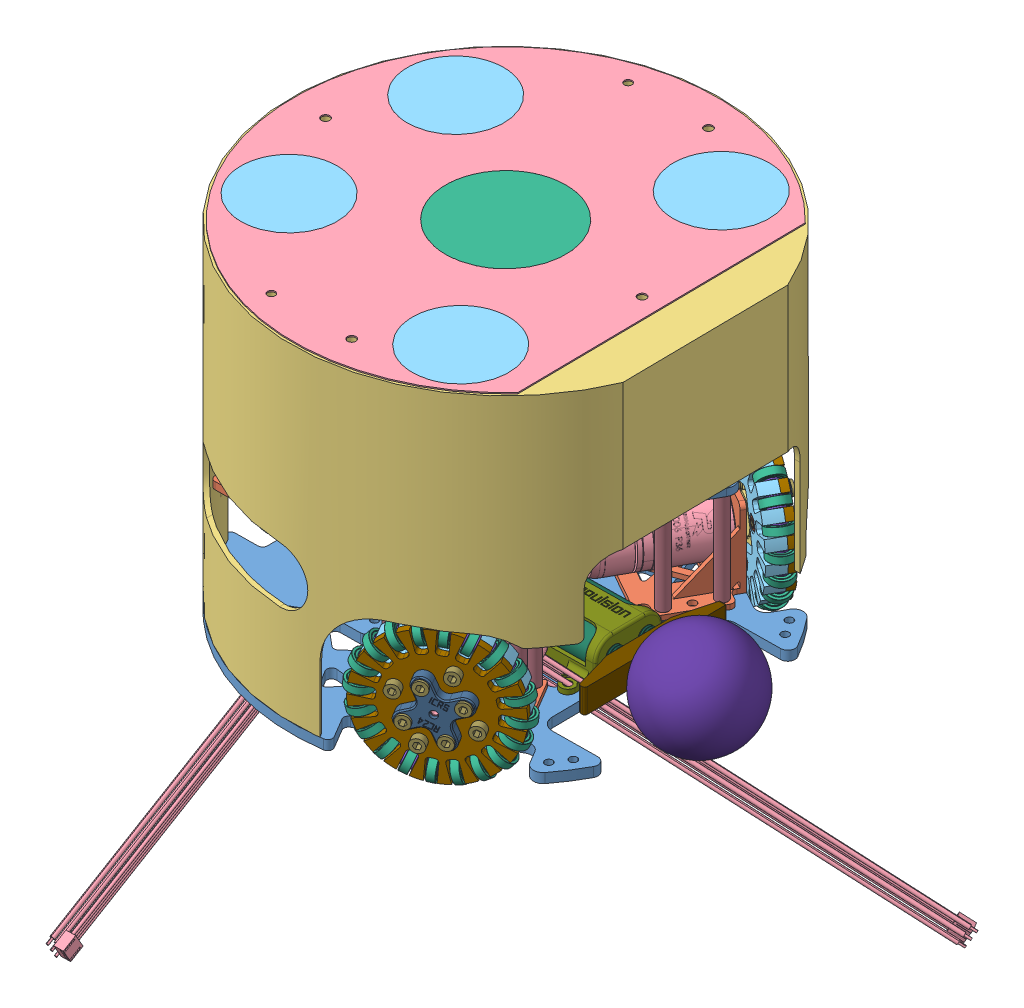
SolidWorks assembly ASM_ICRS_RCssl_2024_drive_base_Tri_wheel-intermediate, configuration Default. Lengths in mm.
Overall size (302.45 245.12 306.72).
392 component instances, 24 part files, 44 mates.
Components (placement in the parent):
- CF4mm_RCssl_drive_base_ground_Tri_wheel-1: CF4mm_RCssl_drive_base_ground_Tri_wheel [Default] at (-0.754 -4 -10.7249) x (-0.011698 0 -0.999932) z (0 1 0) size (182.55 180 57.77)
- RCSSL_gen2_OW_drive_unit-1: RCSSL_gen2_OW_drive_unit [Default] at (35.2509 -22.9667 -96.722) x (0.871815 0 0.489835) z (-0.489835 0 0.871815) size (193.31 168.77 67.31)
  - 1.5mm_aluminium_metal_plating_2006 motor mount-1: 1.5mm_aluminium_metal_plating_2006 motor mount [Default] at (10.7348 39.9667 23.6101) size (46 32 35)
  - 3dp_AL_Gen2_Customised_AL_shaft_flange_connector_2006-1: 3dp_AL_Gen2_Customised_AL_shaft_flange_connector_2006 [Default] at (10.7348 39.9667 8.6101) x (0.866025 0.5 0) z (0 0 1) size (34 34 12.5)
  - RoboMaster M2006 P36 motor 1-1: RoboMaster M2006 P36 motor 1 [默认] at (29.0021 49.1921 55.5053) x (0.258819 0.965926 0) z (0 0 1) size (137.53 138.78 64.81)
  - ASM_RCssl_OW_Ver2-1: ASM_RCssl_OW_Ver2 [Default] at (25.0097 83.9716 -12.1645) x (-0.924615 -0.380903 0) z (0 0 1) size (59.33 59.33 15) (flexible)
    - 3dp_PETG_RCssl_OW_ver2_base-1: 3dp_PETG_RCssl_OW_ver2_base [Default] at (29.9603 35.2502 26.2746) size (54.84 54.84 7)
    - RCssl_OW_Ver2_roller_bearing_ASM-1: RCssl_OW_Ver2_roller_bearing_ASM [Default] at (24.4121 54.6156 21.3003) x (0 1 0) z (1 0 0) size (10 10 6)
      - BK_PU_68_3_10_3_bearing+roller-1: BK_PU_68_3_10_3_bearing+roller [Default] at (5.2981 6.4743 4.0482) size (10 10 3)
      - D3_H6_mid_axis-1: D3_H6_mid_axis [Default] at (5.2981 6.4743 2.5482) size (2.96 2.96 6)
      - m3_D6_H0.5_washer-1: m3_D6_H0.5_washer [Default] at (5.2981 6.4743 3.5482) x (0.872248 -0.489064 0) z (0 0 1) size (6 6 0.5)
      - m3_D6_H0.5_washer-2: m3_D6_H0.5_washer [Default] at (5.2981 6.4743 7.0482) size (6 6 0.5)
    - RCssl_OW_Ver2_roller_bearing_ASM-2: RCssl_OW_Ver2_roller_bearing_ASM [Default] at (30.6679 55.3823 21.3003) x (0.309017 0.951057 0) z (0.951057 -0.309017 0) size (10 10 6)
      - BK_PU_68_3_10_3_bearing+roller-1: BK_PU_68_3_10_3_bearing+roller [Default] at (5.2981 6.4743 4.0482) size (10 10 3)
      - D3_H6_mid_axis-1: D3_H6_mid_axis [Default] at (5.2981 6.4743 2.5482) size (2.96 2.96 6)
      - m3_D6_H0.5_washer-1: m3_D6_H0.5_washer [Default] at (5.2981 6.4743 3.5482) x (0.872248 -0.489064 0) z (0 0 1) size (6 6 0.5)
      - m3_D6_H0.5_washer-2: m3_D6_H0.5_washer [Default] at (5.2981 6.4743 7.0482) size (6 6 0.5)
    - RCssl_OW_Ver2_roller_bearing_ASM-3: RCssl_OW_Ver2_roller_bearing_ASM [Default] at (36.8544 54.1783 21.3003) x (0.587785 0.809017 0) z (0.809017 -0.587785 0) size (10 10 6)
      - BK_PU_68_3_10_3_bearing+roller-1: BK_PU_68_3_10_3_bearing+roller [Default] at (5.2981 6.4743 4.0482) size (10 10 3)
      - D3_H6_mid_axis-1: D3_H6_mid_axis [Default] at (5.2981 6.4743 2.5482) size (2.96 2.96 6)
      - m3_D6_H0.5_washer-1: m3_D6_H0.5_washer [Default] at (5.2981 6.4743 3.5482) x (0.872248 -0.489064 0) z (0 0 1) size (6 6 0.5)
      - m3_D6_H0.5_washer-2: m3_D6_H0.5_washer [Default] at (5.2981 6.4743 7.0482) size (6 6 0.5)
    - RCssl_OW_Ver2_roller_bearing_ASM-4: RCssl_OW_Ver2_roller_bearing_ASM [Default] at (42.3661 51.1215 21.3003) x (0.809017 0.587785 0) z (0.587785 -0.809017 0) size (10 10 6)
      - BK_PU_68_3_10_3_bearing+roller-1: BK_PU_68_3_10_3_bearing+roller [Default] at (5.2981 6.4743 4.0482) size (10 10 3)
      - D3_H6_mid_axis-1: D3_H6_mid_axis [Default] at (5.2981 6.4743 2.5482) size (2.96 2.96 6)
      - m3_D6_H0.5_washer-1: m3_D6_H0.5_washer [Default] at (5.2981 6.4743 3.5482) x (0.872248 -0.489064 0) z (0 0 1) size (6 6 0.5)
      - m3_D6_H0.5_washer-2: m3_D6_H0.5_washer [Default] at (5.2981 6.4743 7.0482) size (6 6 0.5)
    - RCssl_OW_Ver2_roller_bearing_ASM-5: RCssl_OW_Ver2_roller_bearing_ASM [Default] at (46.6634 46.5111 21.3003) x (0.951057 0.309017 0) z (0.309017 -0.951057 0) size (10 10 6)
      - BK_PU_68_3_10_3_bearing+roller-1: BK_PU_68_3_10_3_bearing+roller [Default] at (5.2981 6.4743 4.0482) size (10 10 3)
      - D3_H6_mid_axis-1: D3_H6_mid_axis [Default] at (5.2981 6.4743 2.5482) size (2.96 2.96 6)
      - m3_D6_H0.5_washer-1: m3_D6_H0.5_washer [Default] at (5.2981 6.4743 3.5482) x (0.872248 -0.489064 0) z (0 0 1) size (6 6 0.5)
      - m3_D6_H0.5_washer-2: m3_D6_H0.5_washer [Default] at (5.2981 6.4743 7.0482) size (6 6 0.5)
    - RCssl_OW_Ver2_roller_bearing_ASM-6: RCssl_OW_Ver2_roller_bearing_ASM [Default] at (49.3257 40.7985 21.3003) x (1 0 0) z (0 -1 0) size (10 10 6)
      - BK_PU_68_3_10_3_bearing+roller-1: BK_PU_68_3_10_3_bearing+roller [Default] at (5.2981 6.4743 4.0482) size (10 10 3)
      - D3_H6_mid_axis-1: D3_H6_mid_axis [Default] at (5.2981 6.4743 2.5482) size (2.96 2.96 6)
      - m3_D6_H0.5_washer-1: m3_D6_H0.5_washer [Default] at (5.2981 6.4743 3.5482) x (0.872248 -0.489064 0) z (0 0 1) size (6 6 0.5)
      - m3_D6_H0.5_washer-2: m3_D6_H0.5_washer [Default] at (5.2981 6.4743 7.0482) size (6 6 0.5)
    - RCssl_OW_Ver2_roller_bearing_ASM-7: RCssl_OW_Ver2_roller_bearing_ASM [Default] at (50.0924 34.5427 21.3003) x (0.951057 -0.309017 0) z (-0.309017 -0.951057 0) size (10 10 6)
      - BK_PU_68_3_10_3_bearing+roller-1: BK_PU_68_3_10_3_bearing+roller [Default] at (5.2981 6.4743 4.0482) size (10 10 3)
      - D3_H6_mid_axis-1: D3_H6_mid_axis [Default] at (5.2981 6.4743 2.5482) size (2.96 2.96 6)
      - m3_D6_H0.5_washer-1: m3_D6_H0.5_washer [Default] at (5.2981 6.4743 3.5482) x (0.872248 -0.489064 0) z (0 0 1) size (6 6 0.5)
      - m3_D6_H0.5_washer-2: m3_D6_H0.5_washer [Default] at (5.2981 6.4743 7.0482) size (6 6 0.5)
    - RCssl_OW_Ver2_roller_bearing_ASM-8: RCssl_OW_Ver2_roller_bearing_ASM [Default] at (48.8884 28.3562 21.3003) x (0.809017 -0.587785 0) z (-0.587785 -0.809017 0) size (10 10 6)
      - BK_PU_68_3_10_3_bearing+roller-1: BK_PU_68_3_10_3_bearing+roller [Default] at (5.2981 6.4743 4.0482) size (10 10 3)
      - D3_H6_mid_axis-1: D3_H6_mid_axis [Default] at (5.2981 6.4743 2.5482) size (2.96 2.96 6)
      - m3_D6_H0.5_washer-1: m3_D6_H0.5_washer [Default] at (5.2981 6.4743 3.5482) x (0.872248 -0.489064 0) z (0 0 1) size (6 6 0.5)
      - m3_D6_H0.5_washer-2: m3_D6_H0.5_washer [Default] at (5.2981 6.4743 7.0482) size (6 6 0.5)
    - RCssl_OW_Ver2_roller_bearing_ASM-9: RCssl_OW_Ver2_roller_bearing_ASM [Default] at (45.8316 22.8445 21.3003) x (0.587785 -0.809017 0) z (-0.809017 -0.587785 0) size (10 10 6)
      - BK_PU_68_3_10_3_bearing+roller-1: BK_PU_68_3_10_3_bearing+roller [Default] at (5.2981 6.4743 4.0482) size (10 10 3)
      - D3_H6_mid_axis-1: D3_H6_mid_axis [Default] at (5.2981 6.4743 2.5482) size (2.96 2.96 6)
      - m3_D6_H0.5_washer-1: m3_D6_H0.5_washer [Default] at (5.2981 6.4743 3.5482) x (0.872248 -0.489064 0) z (0 0 1) size (6 6 0.5)
      - m3_D6_H0.5_washer-2: m3_D6_H0.5_washer [Default] at (5.2981 6.4743 7.0482) size (6 6 0.5)
    - RCssl_OW_Ver2_roller_bearing_ASM-10: RCssl_OW_Ver2_roller_bearing_ASM [Default] at (41.2212 18.5472 21.3003) x (0.309017 -0.951057 0) z (-0.951057 -0.309017 0) size (10 10 6)
      - BK_PU_68_3_10_3_bearing+roller-1: BK_PU_68_3_10_3_bearing+roller [Default] at (5.2981 6.4743 4.0482) size (10 10 3)
      - D3_H6_mid_axis-1: D3_H6_mid_axis [Default] at (5.2981 6.4743 2.5482) size (2.96 2.96 6)
      - m3_D6_H0.5_washer-1: m3_D6_H0.5_washer [Default] at (5.2981 6.4743 3.5482) x (0.872248 -0.489064 0) z (0 0 1) size (6 6 0.5)
      - m3_D6_H0.5_washer-2: m3_D6_H0.5_washer [Default] at (5.2981 6.4743 7.0482) size (6 6 0.5)
    - RCssl_OW_Ver2_roller_bearing_ASM-11: RCssl_OW_Ver2_roller_bearing_ASM [Default] at (35.5086 15.8849 21.3003) x (0 -1 0) z (-1 0 0) size (10 10 6)
      - BK_PU_68_3_10_3_bearing+roller-1: BK_PU_68_3_10_3_bearing+roller [Default] at (5.2981 6.4743 4.0482) size (10 10 3)
      - D3_H6_mid_axis-1: D3_H6_mid_axis [Default] at (5.2981 6.4743 2.5482) size (2.96 2.96 6)
      - m3_D6_H0.5_washer-1: m3_D6_H0.5_washer [Default] at (5.2981 6.4743 3.5482) x (0.872248 -0.489064 0) z (0 0 1) size (6 6 0.5)
      - m3_D6_H0.5_washer-2: m3_D6_H0.5_washer [Default] at (5.2981 6.4743 7.0482) size (6 6 0.5)
    - RCssl_OW_Ver2_roller_bearing_ASM-12: RCssl_OW_Ver2_roller_bearing_ASM [Default] at (29.2528 15.1182 21.3003) x (-0.309017 -0.951057 0) z (-0.951057 0.309017 0) size (10 10 6)
      - BK_PU_68_3_10_3_bearing+roller-1: BK_PU_68_3_10_3_bearing+roller [Default] at (5.2981 6.4743 4.0482) size (10 10 3)
      - D3_H6_mid_axis-1: D3_H6_mid_axis [Default] at (5.2981 6.4743 2.5482) size (2.96 2.96 6)
      - m3_D6_H0.5_washer-1: m3_D6_H0.5_washer [Default] at (5.2981 6.4743 3.5482) x (0.872248 -0.489064 0) z (0 0 1) size (6 6 0.5)
      - m3_D6_H0.5_washer-2: m3_D6_H0.5_washer [Default] at (5.2981 6.4743 7.0482) size (6 6 0.5)
    - RCssl_OW_Ver2_roller_bearing_ASM-13: RCssl_OW_Ver2_roller_bearing_ASM [Default] at (23.0663 16.3222 21.3003) x (-0.587785 -0.809017 0) z (-0.809017 0.587785 0) size (10 10 6)
      - BK_PU_68_3_10_3_bearing+roller-1: BK_PU_68_3_10_3_bearing+roller [Default] at (5.2981 6.4743 4.0482) size (10 10 3)
      - D3_H6_mid_axis-1: D3_H6_mid_axis [Default] at (5.2981 6.4743 2.5482) size (2.96 2.96 6)
      - m3_D6_H0.5_washer-1: m3_D6_H0.5_washer [Default] at (5.2981 6.4743 3.5482) x (0.872248 -0.489064 0) z (0 0 1) size (6 6 0.5)
      - m3_D6_H0.5_washer-2: m3_D6_H0.5_washer [Default] at (5.2981 6.4743 7.0482) size (6 6 0.5)
    - RCssl_OW_Ver2_roller_bearing_ASM-14: RCssl_OW_Ver2_roller_bearing_ASM [Default] at (17.5546 19.379 21.3003) x (-0.809017 -0.587785 0) z (-0.587785 0.809017 0) size (10 10 6)
      - BK_PU_68_3_10_3_bearing+roller-1: BK_PU_68_3_10_3_bearing+roller [Default] at (5.2981 6.4743 4.0482) size (10 10 3)
      - D3_H6_mid_axis-1: D3_H6_mid_axis [Default] at (5.2981 6.4743 2.5482) size (2.96 2.96 6)
      - m3_D6_H0.5_washer-1: m3_D6_H0.5_washer [Default] at (5.2981 6.4743 3.5482) x (0.872248 -0.489064 0) z (0 0 1) size (6 6 0.5)
      - m3_D6_H0.5_washer-2: m3_D6_H0.5_washer [Default] at (5.2981 6.4743 7.0482) size (6 6 0.5)
    - RCssl_OW_Ver2_roller_bearing_ASM-15: RCssl_OW_Ver2_roller_bearing_ASM [Default] at (13.2573 23.9893 21.3003) x (-0.951057 -0.309017 0) z (-0.309017 0.951057 0) size (10 10 6)
      - BK_PU_68_3_10_3_bearing+roller-1: BK_PU_68_3_10_3_bearing+roller [Default] at (5.2981 6.4743 4.0482) size (10 10 3)
      - D3_H6_mid_axis-1: D3_H6_mid_axis [Default] at (5.2981 6.4743 2.5482) size (2.96 2.96 6)
      - m3_D6_H0.5_washer-1: m3_D6_H0.5_washer [Default] at (5.2981 6.4743 3.5482) x (0.872248 -0.489064 0) z (0 0 1) size (6 6 0.5)
      - m3_D6_H0.5_washer-2: m3_D6_H0.5_washer [Default] at (5.2981 6.4743 7.0482) size (6 6 0.5)
    - RCssl_OW_Ver2_roller_bearing_ASM-16: RCssl_OW_Ver2_roller_bearing_ASM [Default] at (10.595 29.702 21.3003) x (-1 0 0) z (0 1 0) size (10 10 6)
      - BK_PU_68_3_10_3_bearing+roller-1: BK_PU_68_3_10_3_bearing+roller [Default] at (5.2981 6.4743 4.0482) size (10 10 3)
      - D3_H6_mid_axis-1: D3_H6_mid_axis [Default] at (5.2981 6.4743 2.5482) size (2.96 2.96 6)
      - m3_D6_H0.5_washer-1: m3_D6_H0.5_washer [Default] at (5.2981 6.4743 3.5482) x (0.872248 -0.489064 0) z (0 0 1) size (6 6 0.5)
      - m3_D6_H0.5_washer-2: m3_D6_H0.5_washer [Default] at (5.2981 6.4743 7.0482) size (6 6 0.5)
    - RCssl_OW_Ver2_roller_bearing_ASM-17: RCssl_OW_Ver2_roller_bearing_ASM [Default] at (9.8283 35.9578 21.3003) x (-0.951057 0.309017 0) z (0.309017 0.951057 0) size (10 10 6)
      - BK_PU_68_3_10_3_bearing+roller-1: BK_PU_68_3_10_3_bearing+roller [Default] at (5.2981 6.4743 4.0482) size (10 10 3)
      - D3_H6_mid_axis-1: D3_H6_mid_axis [Default] at (5.2981 6.4743 2.5482) size (2.96 2.96 6)
      - m3_D6_H0.5_washer-1: m3_D6_H0.5_washer [Default] at (5.2981 6.4743 3.5482) x (0.872248 -0.489064 0) z (0 0 1) size (6 6 0.5)
      - m3_D6_H0.5_washer-2: m3_D6_H0.5_washer [Default] at (5.2981 6.4743 7.0482) size (6 6 0.5)
    - RCssl_OW_Ver2_roller_bearing_ASM-18: RCssl_OW_Ver2_roller_bearing_ASM [Default] at (11.0323 42.1443 21.3003) x (-0.809017 0.587785 0) z (0.587785 0.809017 0) size (10 10 6)
      - BK_PU_68_3_10_3_bearing+roller-1: BK_PU_68_3_10_3_bearing+roller [Default] at (5.2981 6.4743 4.0482) size (10 10 3)
      - D3_H6_mid_axis-1: D3_H6_mid_axis [Default] at (5.2981 6.4743 2.5482) size (2.96 2.96 6)
      - m3_D6_H0.5_washer-1: m3_D6_H0.5_washer [Default] at (5.2981 6.4743 3.5482) x (0.872248 -0.489064 0) z (0 0 1) size (6 6 0.5)
      - m3_D6_H0.5_washer-2: m3_D6_H0.5_washer [Default] at (5.2981 6.4743 7.0482) size (6 6 0.5)
    - RCssl_OW_Ver2_roller_bearing_ASM-19: RCssl_OW_Ver2_roller_bearing_ASM [Default] at (14.0891 47.656 21.3003) x (-0.587785 0.809017 0) z (0.809017 0.587785 0) size (10 10 6) (flexible)
      - BK_PU_68_3_10_3_bearing+roller-1: BK_PU_68_3_10_3_bearing+roller [Default] at (5.2981 6.4743 4.0482) size (10 10 3)
      - D3_H6_mid_axis-1: D3_H6_mid_axis [Default] at (5.2981 6.4743 2.5482) size (2.96 2.96 6)
      - m3_D6_H0.5_washer-1: m3_D6_H0.5_washer [Default] at (5.2981 6.4743 3.5482) x (0.872248 -0.489064 0) z (0 0 1) size (6 6 0.5)
      - m3_D6_H0.5_washer-2: m3_D6_H0.5_washer [Default] at (5.2981 6.4743 7.0482) size (6 6 0.5)
    - RCssl_OW_Ver2_roller_bearing_ASM-20: RCssl_OW_Ver2_roller_bearing_ASM [Default] at (18.6994 51.9533 21.3003) x (-0.309017 0.951057 0) z (0.951057 0.309017 0) size (10 10 6)
      - BK_PU_68_3_10_3_bearing+roller-1: BK_PU_68_3_10_3_bearing+roller [Default] at (5.2981 6.4743 4.0482) size (10 10 3)
      - D3_H6_mid_axis-1: D3_H6_mid_axis [Default] at (5.2981 6.4743 2.5482) size (2.96 2.96 6)
      - m3_D6_H0.5_washer-1: m3_D6_H0.5_washer [Default] at (5.2981 6.4743 3.5482) x (0.872248 -0.489064 0) z (0 0 1) size (6 6 0.5)
      - m3_D6_H0.5_washer-2: m3_D6_H0.5_washer [Default] at (5.2981 6.4743 7.0482) size (6 6 0.5)
    - CF3mm_OW_gen2_output_plane-1: CF3mm_OW_gen2_output_plane [Default] at (29.9603 35.2502 44.7746) size (54.84 54.84 3)
    - 3dp_PETG_RCssl_OW_front_lock-1: 3dp_PETG_RCssl_OW_front_lock [Default] at (29.9603 35.2502 21.2746) x (1 0 0) z (0 0 -1) size (21.15 21.15 4.13)
    - nut_din_985-m3x0_5-8-1: nut_din_985-m3x0_5-8 [Default] at (29.9603 21.2502 29.2746) x (-1 0 0) z (0 0 -1) size (6.2 5.5 4)
    - nut_din_985-m3x0_5-8-2: nut_din_985-m3x0_5-8 [Default] at (15.9603 35.2502 29.2746) x (0 1 0) z (0 0 -1) size (6.2 5.5 4)
    - nut_din_985-m3x0_5-8-3: nut_din_985-m3x0_5-8 [Default] at (29.9603 49.2502 29.2746) x (1 0 0) z (0 0 -1) size (6.2 5.5 4)
    - nut_din_985-m3x0_5-8-4: nut_din_985-m3x0_5-8 [Default] at (43.9603 35.2502 29.2746) x (0 -1 0) z (0 0 -1) size (6.2 5.5 4)
    - M3_304__full_teeth__screw_10mm-1: M3_304__full_teeth__screw_10mm [Default] at (29.992 49.2503 23.2746) x (-0.002323 0.999997 0) z (0 0 -1) size (5.3 5.3 13)
    - M3_304__full_teeth__screw_10mm-2: M3_304__full_teeth__screw_10mm [Default] at (43.9604 35.2186 23.2746) x (0.999997 0.002323 0) z (0 0 -1) size (5.3 5.3 13)
    - M3_304__full_teeth__screw_10mm-3: M3_304__full_teeth__screw_10mm [Default] at (29.9287 21.2502 23.2746) x (0.002323 -0.999997 0) z (0 0 -1) size (5.3 5.3 13)
    - M3_304__full_teeth__screw_10mm-4: M3_304__full_teeth__screw_10mm [Default] at (15.9603 35.2819 23.2746) x (-0.999997 -0.002323 0) z (0 0 -1) size (5.3 5.3 13)
    - M3_304__full_teeth__screw_10mm-5: M3_304__full_teeth__screw_10mm [Default] at (37.0442 42.2923 21.2746) x (0.914728 0.40407 0) z (0 0 -1) size (5.3 5.3 13)
    - M3_304__full_teeth__screw_10mm-6: M3_304__full_teeth__screw_10mm [Default] at (37.0024 28.1664 21.2746) x (0.40407 -0.914728 0) z (0 0 -1) size (5.3 5.3 13)
    - M3_304__full_teeth__screw_10mm-7: M3_304__full_teeth__screw_10mm [Default] at (22.8765 28.2081 21.2746) x (-0.914728 -0.40407 0) z (0 0 -1) size (5.3 5.3 13)
    - M3_304__full_teeth__screw_10mm-8: M3_304__full_teeth__screw_10mm [Default] at (22.9182 42.3341 21.2746) x (-0.40407 0.914728 0) z (0 0 -1) size (5.3 5.3 13)
  - AL_pillar_M3_D6_H40_Threaded-2: AL_pillar_M3_D6_H40_Threaded [H30] at (-8.7652 24.9667 50.1101) size (5 40 5)
  - AL_pillar_M3_D6_H40_Threaded-3: AL_pillar_M3_D6_H40_Threaded [H30] at (30.2348 24.9667 50.1101) size (5 40 5)
  - AL_pillar_M3_D6_H40_Threaded-4: AL_pillar_M3_D6_H40_Threaded [Default] at (30.2348 24.9667 32.1101) x (0.546545 0 0.83743) z (-0.83743 0 0.546545) size (5 40 5)
  - AL_pillar_M3_D6_H40_Threaded-5: AL_pillar_M3_D6_H40_Threaded [Default] at (-8.7652 24.9667 32.1101) x (0.546545 0 0.83743) z (-0.83743 0 0.546545) size (5 40 5)
- RCSSL_gen2_OW_drive_unit-2: RCSSL_gen2_OW_drive_unit [Default] at (55.7193 -22.9667 63.4549) x (-0.860117 0 0.510097) z (-0.510097 0 -0.860117) size (193.31 168.77 67.31)
  - 1.5mm_aluminium_metal_plating_2006 motor mount-1: 1.5mm_aluminium_metal_plating_2006 motor mount [Default] at (10.7348 39.9667 23.6101) size (46 32 35)
  - 3dp_AL_Gen2_Customised_AL_shaft_flange_connector_2006-1: 3dp_AL_Gen2_Customised_AL_shaft_flange_connector_2006 [Default] at (10.7348 39.9667 8.6101) x (0.866025 0.5 0) z (0 0 1) size (34 34 12.5)
  - RoboMaster M2006 P36 motor 1-1: RoboMaster M2006 P36 motor 1 [默认] at (29.0021 49.1921 55.5053) x (0.258819 0.965926 0) z (0 0 1) size (137.53 138.78 64.81)
  - ASM_RCssl_OW_Ver2-1: ASM_RCssl_OW_Ver2 [Default] at (25.0097 83.9716 -12.1645) x (-0.924615 -0.380903 0) z (0 0 1) size (59.33 59.33 15) (flexible)
    - 3dp_PETG_RCssl_OW_ver2_base-1: 3dp_PETG_RCssl_OW_ver2_base [Default] at (29.9603 35.2502 26.2746) size (54.84 54.84 7)
    - RCssl_OW_Ver2_roller_bearing_ASM-1: RCssl_OW_Ver2_roller_bearing_ASM [Default] at (24.4121 54.6156 21.3003) x (0 1 0) z (1 0 0) size (10 10 6)
      - BK_PU_68_3_10_3_bearing+roller-1: BK_PU_68_3_10_3_bearing+roller [Default] at (5.2981 6.4743 4.0482) size (10 10 3)
      - D3_H6_mid_axis-1: D3_H6_mid_axis [Default] at (5.2981 6.4743 2.5482) size (2.96 2.96 6)
      - m3_D6_H0.5_washer-1: m3_D6_H0.5_washer [Default] at (5.2981 6.4743 3.5482) x (0.872248 -0.489064 0) z (0 0 1) size (6 6 0.5)
      - m3_D6_H0.5_washer-2: m3_D6_H0.5_washer [Default] at (5.2981 6.4743 7.0482) size (6 6 0.5)
    - RCssl_OW_Ver2_roller_bearing_ASM-2: RCssl_OW_Ver2_roller_bearing_ASM [Default] at (30.6679 55.3823 21.3003) x (0.309017 0.951057 0) z (0.951057 -0.309017 0) size (10 10 6)
      - BK_PU_68_3_10_3_bearing+roller-1: BK_PU_68_3_10_3_bearing+roller [Default] at (5.2981 6.4743 4.0482) size (10 10 3)
      - D3_H6_mid_axis-1: D3_H6_mid_axis [Default] at (5.2981 6.4743 2.5482) size (2.96 2.96 6)
      - m3_D6_H0.5_washer-1: m3_D6_H0.5_washer [Default] at (5.2981 6.4743 3.5482) x (0.872248 -0.489064 0) z (0 0 1) size (6 6 0.5)
      - m3_D6_H0.5_washer-2: m3_D6_H0.5_washer [Default] at (5.2981 6.4743 7.0482) size (6 6 0.5)
    - RCssl_OW_Ver2_roller_bearing_ASM-3: RCssl_OW_Ver2_roller_bearing_ASM [Default] at (36.8544 54.1783 21.3003) x (0.587785 0.809017 0) z (0.809017 -0.587785 0) size (10 10 6)
      - BK_PU_68_3_10_3_bearing+roller-1: BK_PU_68_3_10_3_bearing+roller [Default] at (5.2981 6.4743 4.0482) size (10 10 3)
      - D3_H6_mid_axis-1: D3_H6_mid_axis [Default] at (5.2981 6.4743 2.5482) size (2.96 2.96 6)
      - m3_D6_H0.5_washer-1: m3_D6_H0.5_washer [Default] at (5.2981 6.4743 3.5482) x (0.872248 -0.489064 0) z (0 0 1) size (6 6 0.5)
      - m3_D6_H0.5_washer-2: m3_D6_H0.5_washer [Default] at (5.2981 6.4743 7.0482) size (6 6 0.5)
    - RCssl_OW_Ver2_roller_bearing_ASM-4: RCssl_OW_Ver2_roller_bearing_ASM [Default] at (42.3661 51.1215 21.3003) x (0.809017 0.587785 0) z (0.587785 -0.809017 0) size (10 10 6)
      - BK_PU_68_3_10_3_bearing+roller-1: BK_PU_68_3_10_3_bearing+roller [Default] at (5.2981 6.4743 4.0482) size (10 10 3)
      - D3_H6_mid_axis-1: D3_H6_mid_axis [Default] at (5.2981 6.4743 2.5482) size (2.96 2.96 6)
      - m3_D6_H0.5_washer-1: m3_D6_H0.5_washer [Default] at (5.2981 6.4743 3.5482) x (0.872248 -0.489064 0) z (0 0 1) size (6 6 0.5)
      - m3_D6_H0.5_washer-2: m3_D6_H0.5_washer [Default] at (5.2981 6.4743 7.0482) size (6 6 0.5)
    - RCssl_OW_Ver2_roller_bearing_ASM-5: RCssl_OW_Ver2_roller_bearing_ASM [Default] at (46.6634 46.5111 21.3003) x (0.951057 0.309017 0) z (0.309017 -0.951057 0) size (10 10 6)
      - BK_PU_68_3_10_3_bearing+roller-1: BK_PU_68_3_10_3_bearing+roller [Default] at (5.2981 6.4743 4.0482) size (10 10 3)
      - D3_H6_mid_axis-1: D3_H6_mid_axis [Default] at (5.2981 6.4743 2.5482) size (2.96 2.96 6)
      - m3_D6_H0.5_washer-1: m3_D6_H0.5_washer [Default] at (5.2981 6.4743 3.5482) x (0.872248 -0.489064 0) z (0 0 1) size (6 6 0.5)
      - m3_D6_H0.5_washer-2: m3_D6_H0.5_washer [Default] at (5.2981 6.4743 7.0482) size (6 6 0.5)
    - RCssl_OW_Ver2_roller_bearing_ASM-6: RCssl_OW_Ver2_roller_bearing_ASM [Default] at (49.3257 40.7985 21.3003) x (1 0 0) z (0 -1 0) size (10 10 6)
      - BK_PU_68_3_10_3_bearing+roller-1: BK_PU_68_3_10_3_bearing+roller [Default] at (5.2981 6.4743 4.0482) size (10 10 3)
      - D3_H6_mid_axis-1: D3_H6_mid_axis [Default] at (5.2981 6.4743 2.5482) size (2.96 2.96 6)
      - m3_D6_H0.5_washer-1: m3_D6_H0.5_washer [Default] at (5.2981 6.4743 3.5482) x (0.872248 -0.489064 0) z (0 0 1) size (6 6 0.5)
      - m3_D6_H0.5_washer-2: m3_D6_H0.5_washer [Default] at (5.2981 6.4743 7.0482) size (6 6 0.5)
    - RCssl_OW_Ver2_roller_bearing_ASM-7: RCssl_OW_Ver2_roller_bearing_ASM [Default] at (50.0924 34.5427 21.3003) x (0.951057 -0.309017 0) z (-0.309017 -0.951057 0) size (10 10 6)
      - BK_PU_68_3_10_3_bearing+roller-1: BK_PU_68_3_10_3_bearing+roller [Default] at (5.2981 6.4743 4.0482) size (10 10 3)
      - D3_H6_mid_axis-1: D3_H6_mid_axis [Default] at (5.2981 6.4743 2.5482) size (2.96 2.96 6)
      - m3_D6_H0.5_washer-1: m3_D6_H0.5_washer [Default] at (5.2981 6.4743 3.5482) x (0.872248 -0.489064 0) z (0 0 1) size (6 6 0.5)
      - m3_D6_H0.5_washer-2: m3_D6_H0.5_washer [Default] at (5.2981 6.4743 7.0482) size (6 6 0.5)
    - RCssl_OW_Ver2_roller_bearing_ASM-8: RCssl_OW_Ver2_roller_bearing_ASM [Default] at (48.8884 28.3562 21.3003) x (0.809017 -0.587785 0) z (-0.587785 -0.809017 0) size (10 10 6)
      - BK_PU_68_3_10_3_bearing+roller-1: BK_PU_68_3_10_3_bearing+roller [Default] at (5.2981 6.4743 4.0482) size (10 10 3)
      - D3_H6_mid_axis-1: D3_H6_mid_axis [Default] at (5.2981 6.4743 2.5482) size (2.96 2.96 6)
      - m3_D6_H0.5_washer-1: m3_D6_H0.5_washer [Default] at (5.2981 6.4743 3.5482) x (0.872248 -0.489064 0) z (0 0 1) size (6 6 0.5)
      - m3_D6_H0.5_washer-2: m3_D6_H0.5_washer [Default] at (5.2981 6.4743 7.0482) size (6 6 0.5)
    - RCssl_OW_Ver2_roller_bearing_ASM-9: RCssl_OW_Ver2_roller_bearing_ASM [Default] at (45.8316 22.8445 21.3003) x (0.587785 -0.809017 0) z (-0.809017 -0.587785 0) size (10 10 6)
      - BK_PU_68_3_10_3_bearing+roller-1: BK_PU_68_3_10_3_bearing+roller [Default] at (5.2981 6.4743 4.0482) size (10 10 3)
      - D3_H6_mid_axis-1: D3_H6_mid_axis [Default] at (5.2981 6.4743 2.5482) size (2.96 2.96 6)
      - m3_D6_H0.5_washer-1: m3_D6_H0.5_washer [Default] at (5.2981 6.4743 3.5482) x (0.872248 -0.489064 0) z (0 0 1) size (6 6 0.5)
      - m3_D6_H0.5_washer-2: m3_D6_H0.5_washer [Default] at (5.2981 6.4743 7.0482) size (6 6 0.5)
    - RCssl_OW_Ver2_roller_bearing_ASM-10: RCssl_OW_Ver2_roller_bearing_ASM [Default] at (41.2212 18.5472 21.3003) x (0.309017 -0.951057 0) z (-0.951057 -0.309017 0) size (10 10 6)
      - BK_PU_68_3_10_3_bearing+roller-1: BK_PU_68_3_10_3_bearing+roller [Default] at (5.2981 6.4743 4.0482) size (10 10 3)
      - D3_H6_mid_axis-1: D3_H6_mid_axis [Default] at (5.2981 6.4743 2.5482) size (2.96 2.96 6)
      - m3_D6_H0.5_washer-1: m3_D6_H0.5_washer [Default] at (5.2981 6.4743 3.5482) x (0.872248 -0.489064 0) z (0 0 1) size (6 6 0.5)
      - m3_D6_H0.5_washer-2: m3_D6_H0.5_washer [Default] at (5.2981 6.4743 7.0482) size (6 6 0.5)
    - RCssl_OW_Ver2_roller_bearing_ASM-11: RCssl_OW_Ver2_roller_bearing_ASM [Default] at (35.5086 15.8849 21.3003) x (0 -1 0) z (-1 0 0) size (10 10 6)
      - BK_PU_68_3_10_3_bearing+roller-1: BK_PU_68_3_10_3_bearing+roller [Default] at (5.2981 6.4743 4.0482) size (10 10 3)
      - D3_H6_mid_axis-1: D3_H6_mid_axis [Default] at (5.2981 6.4743 2.5482) size (2.96 2.96 6)
      - m3_D6_H0.5_washer-1: m3_D6_H0.5_washer [Default] at (5.2981 6.4743 3.5482) x (0.872248 -0.489064 0) z (0 0 1) size (6 6 0.5)
      - m3_D6_H0.5_washer-2: m3_D6_H0.5_washer [Default] at (5.2981 6.4743 7.0482) size (6 6 0.5)
    - RCssl_OW_Ver2_roller_bearing_ASM-12: RCssl_OW_Ver2_roller_bearing_ASM [Default] at (29.2528 15.1182 21.3003) x (-0.309017 -0.951057 0) z (-0.951057 0.309017 0) size (10 10 6)
      - BK_PU_68_3_10_3_bearing+roller-1: BK_PU_68_3_10_3_bearing+roller [Default] at (5.2981 6.4743 4.0482) size (10 10 3)
      - D3_H6_mid_axis-1: D3_H6_mid_axis [Default] at (5.2981 6.4743 2.5482) size (2.96 2.96 6)
      - m3_D6_H0.5_washer-1: m3_D6_H0.5_washer [Default] at (5.2981 6.4743 3.5482) x (0.872248 -0.489064 0) z (0 0 1) size (6 6 0.5)
      - m3_D6_H0.5_washer-2: m3_D6_H0.5_washer [Default] at (5.2981 6.4743 7.0482) size (6 6 0.5)
    - RCssl_OW_Ver2_roller_bearing_ASM-13: RCssl_OW_Ver2_roller_bearing_ASM [Default] at (23.0663 16.3222 21.3003) x (-0.587785 -0.809017 0) z (-0.809017 0.587785 0) size (10 10 6)
      - BK_PU_68_3_10_3_bearing+roller-1: BK_PU_68_3_10_3_bearing+roller [Default] at (5.2981 6.4743 4.0482) size (10 10 3)
      - D3_H6_mid_axis-1: D3_H6_mid_axis [Default] at (5.2981 6.4743 2.5482) size (2.96 2.96 6)
      - m3_D6_H0.5_washer-1: m3_D6_H0.5_washer [Default] at (5.2981 6.4743 3.5482) x (0.872248 -0.489064 0) z (0 0 1) size (6 6 0.5)
      - m3_D6_H0.5_washer-2: m3_D6_H0.5_washer [Default] at (5.2981 6.4743 7.0482) size (6 6 0.5)
    - RCssl_OW_Ver2_roller_bearing_ASM-14: RCssl_OW_Ver2_roller_bearing_ASM [Default] at (17.5546 19.379 21.3003) x (-0.809017 -0.587785 0) z (-0.587785 0.809017 0) size (10 10 6)
      - BK_PU_68_3_10_3_bearing+roller-1: BK_PU_68_3_10_3_bearing+roller [Default] at (5.2981 6.4743 4.0482) size (10 10 3)
      - D3_H6_mid_axis-1: D3_H6_mid_axis [Default] at (5.2981 6.4743 2.5482) size (2.96 2.96 6)
      - m3_D6_H0.5_washer-1: m3_D6_H0.5_washer [Default] at (5.2981 6.4743 3.5482) x (0.872248 -0.489064 0) z (0 0 1) size (6 6 0.5)
      - m3_D6_H0.5_washer-2: m3_D6_H0.5_washer [Default] at (5.2981 6.4743 7.0482) size (6 6 0.5)
    - RCssl_OW_Ver2_roller_bearing_ASM-15: RCssl_OW_Ver2_roller_bearing_ASM [Default] at (13.2573 23.9893 21.3003) x (-0.951057 -0.309017 0) z (-0.309017 0.951057 0) size (10 10 6)
      - BK_PU_68_3_10_3_bearing+roller-1: BK_PU_68_3_10_3_bearing+roller [Default] at (5.2981 6.4743 4.0482) size (10 10 3)
      - D3_H6_mid_axis-1: D3_H6_mid_axis [Default] at (5.2981 6.4743 2.5482) size (2.96 2.96 6)
      - m3_D6_H0.5_washer-1: m3_D6_H0.5_washer [Default] at (5.2981 6.4743 3.5482) x (0.872248 -0.489064 0) z (0 0 1) size (6 6 0.5)
      - m3_D6_H0.5_washer-2: m3_D6_H0.5_washer [Default] at (5.2981 6.4743 7.0482) size (6 6 0.5)
    - RCssl_OW_Ver2_roller_bearing_ASM-16: RCssl_OW_Ver2_roller_bearing_ASM [Default] at (10.595 29.702 21.3003) x (-1 0 0) z (0 1 0) size (10 10 6)
      - BK_PU_68_3_10_3_bearing+roller-1: BK_PU_68_3_10_3_bearing+roller [Default] at (5.2981 6.4743 4.0482) size (10 10 3)
      - D3_H6_mid_axis-1: D3_H6_mid_axis [Default] at (5.2981 6.4743 2.5482) size (2.96 2.96 6)
      - m3_D6_H0.5_washer-1: m3_D6_H0.5_washer [Default] at (5.2981 6.4743 3.5482) x (0.872248 -0.489064 0) z (0 0 1) size (6 6 0.5)
      - m3_D6_H0.5_washer-2: m3_D6_H0.5_washer [Default] at (5.2981 6.4743 7.0482) size (6 6 0.5)
    - RCssl_OW_Ver2_roller_bearing_ASM-17: RCssl_OW_Ver2_roller_bearing_ASM [Default] at (9.8283 35.9578 21.3003) x (-0.951057 0.309017 0) z (0.309017 0.951057 0) size (10 10 6)
      - BK_PU_68_3_10_3_bearing+roller-1: BK_PU_68_3_10_3_bearing+roller [Default] at (5.2981 6.4743 4.0482) size (10 10 3)
      - D3_H6_mid_axis-1: D3_H6_mid_axis [Default] at (5.2981 6.4743 2.5482) size (2.96 2.96 6)
      - m3_D6_H0.5_washer-1: m3_D6_H0.5_washer [Default] at (5.2981 6.4743 3.5482) x (0.872248 -0.489064 0) z (0 0 1) size (6 6 0.5)
      - m3_D6_H0.5_washer-2: m3_D6_H0.5_washer [Default] at (5.2981 6.4743 7.0482) size (6 6 0.5)
    - RCssl_OW_Ver2_roller_bearing_ASM-18: RCssl_OW_Ver2_roller_bearing_ASM [Default] at (11.0323 42.1443 21.3003) x (-0.809017 0.587785 0) z (0.587785 0.809017 0) size (10 10 6)
      - BK_PU_68_3_10_3_bearing+roller-1: BK_PU_68_3_10_3_bearing+roller [Default] at (5.2981 6.4743 4.0482) size (10 10 3)
      - D3_H6_mid_axis-1: D3_H6_mid_axis [Default] at (5.2981 6.4743 2.5482) size (2.96 2.96 6)
      - m3_D6_H0.5_washer-1: m3_D6_H0.5_washer [Default] at (5.2981 6.4743 3.5482) x (0.872248 -0.489064 0) z (0 0 1) size (6 6 0.5)
      - m3_D6_H0.5_washer-2: m3_D6_H0.5_washer [Default] at (5.2981 6.4743 7.0482) size (6 6 0.5)
    - RCssl_OW_Ver2_roller_bearing_ASM-19: RCssl_OW_Ver2_roller_bearing_ASM [Default] at (14.0891 47.656 21.3003) x (-0.587785 0.809017 0) z (0.809017 0.587785 0) size (10 10 6) (flexible)
      - BK_PU_68_3_10_3_bearing+roller-1: BK_PU_68_3_10_3_bearing+roller [Default] at (5.2981 6.4743 4.0482) size (10 10 3)
      - D3_H6_mid_axis-1: D3_H6_mid_axis [Default] at (5.2981 6.4743 2.5482) size (2.96 2.96 6)
      - m3_D6_H0.5_washer-1: m3_D6_H0.5_washer [Default] at (5.2981 6.4743 3.5482) x (0.872248 -0.489064 0) z (0 0 1) size (6 6 0.5)
      - m3_D6_H0.5_washer-2: m3_D6_H0.5_washer [Default] at (5.2981 6.4743 7.0482) size (6 6 0.5)
    - RCssl_OW_Ver2_roller_bearing_ASM-20: RCssl_OW_Ver2_roller_bearing_ASM [Default] at (18.6994 51.9533 21.3003) x (-0.309017 0.951057 0) z (0.951057 0.309017 0) size (10 10 6)
      - BK_PU_68_3_10_3_bearing+roller-1: BK_PU_68_3_10_3_bearing+roller [Default] at (5.2981 6.4743 4.0482) size (10 10 3)
      - D3_H6_mid_axis-1: D3_H6_mid_axis [Default] at (5.2981 6.4743 2.5482) size (2.96 2.96 6)
      - m3_D6_H0.5_washer-1: m3_D6_H0.5_washer [Default] at (5.2981 6.4743 3.5482) x (0.872248 -0.489064 0) z (0 0 1) size (6 6 0.5)
      - m3_D6_H0.5_washer-2: m3_D6_H0.5_washer [Default] at (5.2981 6.4743 7.0482) size (6 6 0.5)
    - CF3mm_OW_gen2_output_plane-1: CF3mm_OW_gen2_output_plane [Default] at (29.9603 35.2502 44.7746) size (54.84 54.84 3)
    - 3dp_PETG_RCssl_OW_front_lock-1: 3dp_PETG_RCssl_OW_front_lock [Default] at (29.9603 35.2502 21.2746) x (1 0 0) z (0 0 -1) size (21.15 21.15 4.13)
    - nut_din_985-m3x0_5-8-1: nut_din_985-m3x0_5-8 [Default] at (29.9603 21.2502 29.2746) x (-1 0 0) z (0 0 -1) size (6.2 5.5 4)
    - nut_din_985-m3x0_5-8-2: nut_din_985-m3x0_5-8 [Default] at (15.9603 35.2502 29.2746) x (0 1 0) z (0 0 -1) size (6.2 5.5 4)
    - nut_din_985-m3x0_5-8-3: nut_din_985-m3x0_5-8 [Default] at (29.9603 49.2502 29.2746) x (1 0 0) z (0 0 -1) size (6.2 5.5 4)
    - nut_din_985-m3x0_5-8-4: nut_din_985-m3x0_5-8 [Default] at (43.9603 35.2502 29.2746) x (0 -1 0) z (0 0 -1) size (6.2 5.5 4)
    - M3_304__full_teeth__screw_10mm-1: M3_304__full_teeth__screw_10mm [Default] at (29.992 49.2503 23.2746) x (-0.002323 0.999997 0) z (0 0 -1) size (5.3 5.3 13)
    - M3_304__full_teeth__screw_10mm-2: M3_304__full_teeth__screw_10mm [Default] at (43.9604 35.2186 23.2746) x (0.999997 0.002323 0) z (0 0 -1) size (5.3 5.3 13)
    - M3_304__full_teeth__screw_10mm-3: M3_304__full_teeth__screw_10mm [Default] at (29.9287 21.2502 23.2746) x (0.002323 -0.999997 0) z (0 0 -1) size (5.3 5.3 13)
    - M3_304__full_teeth__screw_10mm-4: M3_304__full_teeth__screw_10mm [Default] at (15.9603 35.2819 23.2746) x (-0.999997 -0.002323 0) z (0 0 -1) size (5.3 5.3 13)
    - M3_304__full_teeth__screw_10mm-5: M3_304__full_teeth__screw_10mm [Default] at (37.0442 42.2923 21.2746) x (0.914728 0.40407 0) z (0 0 -1) size (5.3 5.3 13)
    - M3_304__full_teeth__screw_10mm-6: M3_304__full_teeth__screw_10mm [Default] at (37.0024 28.1664 21.2746) x (0.40407 -0.914728 0) z (0 0 -1) size (5.3 5.3 13)
    - M3_304__full_teeth__screw_10mm-7: M3_304__full_teeth__screw_10mm [Default] at (22.8765 28.2081 21.2746) x (-0.914728 -0.40407 0) z (0 0 -1) size (5.3 5.3 13)
    - M3_304__full_teeth__screw_10mm-8: M3_304__full_teeth__screw_10mm [Default] at (22.9182 42.3341 21.2746) x (-0.40407 0.914728 0) z (0 0 -1) size (5.3 5.3 13)
  - AL_pillar_M3_D6_H40_Threaded-2: AL_pillar_M3_D6_H40_Threaded [H30] at (-8.7652 24.9667 50.1101) size (5 40 5)
  - AL_pillar_M3_D6_H40_Threaded-3: AL_pillar_M3_D6_H40_Threaded [H30] at (30.2348 24.9667 50.1101) size (5 40 5)
  - AL_pillar_M3_D6_H40_Threaded-4: AL_pillar_M3_D6_H40_Threaded [Default] at (30.2348 24.9667 32.1101) x (0.546545 0 0.83743) z (-0.83743 0 0.546545) size (5 40 5)
  - AL_pillar_M3_D6_H40_Threaded-5: AL_pillar_M3_D6_H40_Threaded [Default] at (-8.7652 24.9667 32.1101) x (0.546545 0 0.83743) z (-0.83743 0 0.546545) size (5 40 5)
